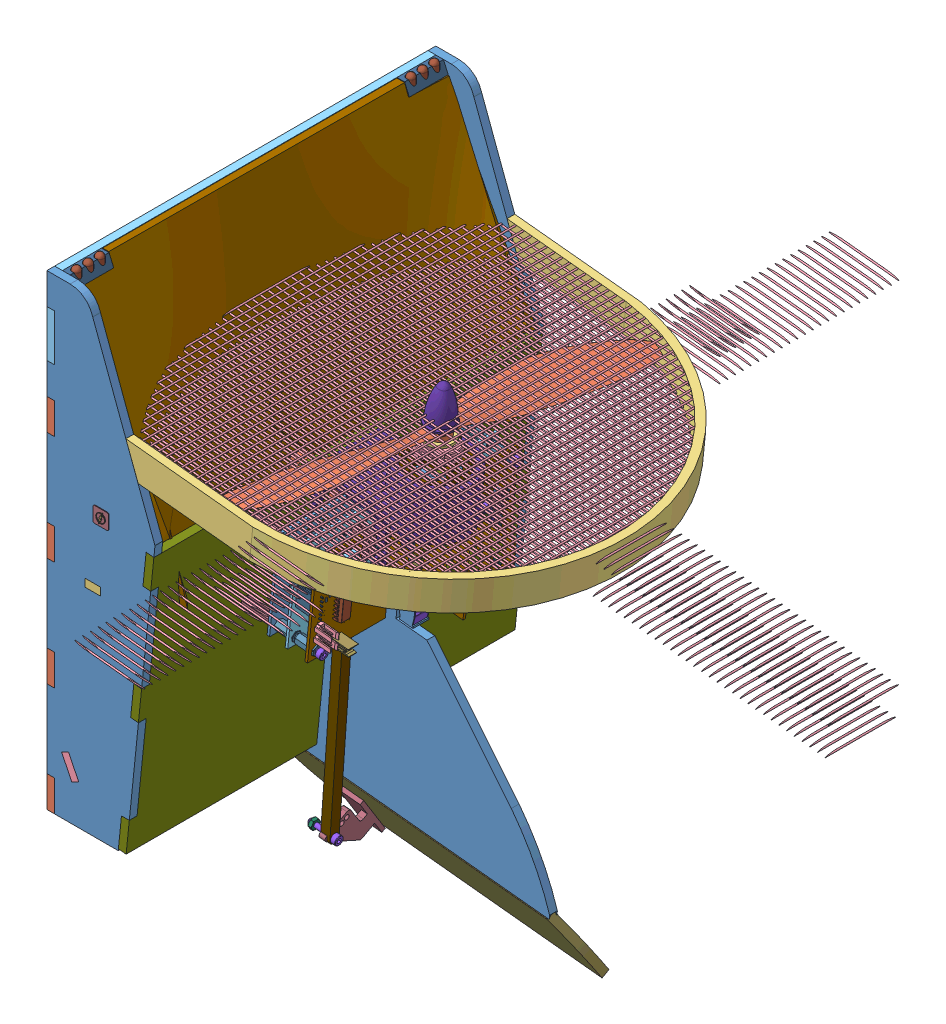
SolidWorks assembly AssTotaleSimu3, configuration Défaut. Lengths in mm. (continued)
Components (placement in the parent): (continued)
- AssStructSimu-1: AssStructSimu [Défaut] at (-125.7658 -1.8483 624.6548) x (1 0 0) z (0 0 -1) size (253.25 324.59 251.6) (continued)
  - AssCarte-1: AssCarte [Défaut] at (38.0121 147.1029 290.772) x (-0.101852 0.9948 0) z (0.9948 0.101852 0) size (66.52 130.57 98.72) (continued)
    - AssEntretoise-3: AssEntretoise [Défaut] at (-106.8199 -51.2976 37.1344) x (0 0 -1) z (1 0 0) size (58.24 7.29 7.81)
      - socket head cap screw 4762_din-1: socket head cap screw 4762_din [EN ISO 4762 M3 x 5 - 5N] at (-2.4967 0.5867 0) size (8 5.5 5.5)
      - hexagonal_spacer_MF_M3_H20_HEX5.5_FTD6_MTL6-1: hexagonal_spacer_MF_M3_H20_HEX5.5_FTD6_MTL6 [Défaut] at (48.3433 0.5867 0) x (0 0 1) z (-1 0 0) size (6.36 5.51 26)
      - hex nut style 1 gradeab_din-1: hex nut style 1 gradeab_din [Hexagon Nut ISO 4032 - M3 - W - N] at (53.3433 0.5867 0) x (0 0.943962 0.330053) z (-1 0 0) size (5.5 6.35 2.4)
      - hexagonal_spacer_MF_M3_H12_HEX5.5_FTD6_MTL6-2: hexagonal_spacer_MF_M3_H12_HEX5.5_FTD6_MTL6 [Défaut] at (27.0633 0.5867 0) x (0 0.248308 0.968681) z (-1 0 0) size (6.36 5.51 18)
      - hexagonal_spacer_MF_M3_H12_HEX5.5_FTD6_MTL6-3: hexagonal_spacer_MF_M3_H12_HEX5.5_FTD6_MTL6 [Défaut] at (13.7833 0.5867 0) x (0 0 1) z (-1 0 0) size (6.36 5.51 18)
    - AssEntretoise-4: AssEntretoise [Défaut] at (-106.8199 68.7024 37.1344) x (0 0 -1) z (1 0 0) size (58.24 7.29 7.81)
      - socket head cap screw 4762_din-1: socket head cap screw 4762_din [EN ISO 4762 M3 x 5 - 5N] at (-2.4967 0.5867 0) size (8 5.5 5.5)
      - hexagonal_spacer_MF_M3_H20_HEX5.5_FTD6_MTL6-1: hexagonal_spacer_MF_M3_H20_HEX5.5_FTD6_MTL6 [Défaut] at (48.3433 0.5867 0) x (0 0 1) z (-1 0 0) size (6.36 5.51 26)
      - hex nut style 1 gradeab_din-1: hex nut style 1 gradeab_din [Hexagon Nut ISO 4032 - M3 - W - N] at (53.3433 0.5867 0) x (0 0.943962 0.330053) z (-1 0 0) size (5.5 6.35 2.4)
      - hexagonal_spacer_MF_M3_H12_HEX5.5_FTD6_MTL6-2: hexagonal_spacer_MF_M3_H12_HEX5.5_FTD6_MTL6 [Défaut] at (27.0633 0.5867 0) x (0 0.248308 0.968681) z (-1 0 0) size (6.36 5.51 18)
      - hexagonal_spacer_MF_M3_H12_HEX5.5_FTD6_MTL6-3: hexagonal_spacer_MF_M3_H12_HEX5.5_FTD6_MTL6 [Défaut] at (13.7833 0.5867 0) x (0 0 1) z (-1 0 0) size (6.36 5.51 18)
    - AssMpu-1: AssMpu [Défaut] at (-150.6881 40.5798 29.6372) x (0.908747 0.417347 0) z (0 0 1) size (8 8 22.28)
      - hex nut style 1 gradeab_din-1: hex nut style 1 gradeab_din [Hexagon Nut ISO 4032 - M3 - W - N] at (0.2783 0.3227 1.2) size (5.5 6.35 2.4)
      - plain washer 6903 type ab_din-1: plain washer 6903 type ab_din [DIN 6903-A3] at (0.2783 0.3227 1.2) x (0 0 1) z (-1 0 0) size (1 8 8)
      - socket head cap screw 4762_din-1: socket head cap screw 4762_din [EN ISO 4762 M3 x 5 - 5N] at (0.2783 0.3227 19.76) x (0 0 -1) z (-0.852155 0.523289 0) size (8 5.5 5.5)
      - hexagonal_spacer_MF_M3_H12_HEX5.5_FTD6_MTL6-1: hexagonal_spacer_MF_M3_H12_HEX5.5_FTD6_MTL6 [Défaut] at (0.2783 0.3227 3.48) size (6.36 5.51 18)
    - AssMpu-2: AssMpu [Défaut] at (-130.3481 40.6665 29.6372) size (8 8 22.28)
      - hex nut style 1 gradeab_din-1: hex nut style 1 gradeab_din [Hexagon Nut ISO 4032 - M3 - W - N] at (0.2783 0.3227 1.2) size (5.5 6.35 2.4)
      - plain washer 6903 type ab_din-1: plain washer 6903 type ab_din [DIN 6903-A3] at (0.2783 0.3227 1.2) x (0 0 1) z (-1 0 0) size (1 8 8)
      - socket head cap screw 4762_din-1: socket head cap screw 4762_din [EN ISO 4762 M3 x 5 - 5N] at (0.2783 0.3227 19.76) x (0 0 -1) z (-0.852155 0.523289 0) size (8 5.5 5.5)
      - hexagonal_spacer_MF_M3_H12_HEX5.5_FTD6_MTL6-1: hexagonal_spacer_MF_M3_H12_HEX5.5_FTD6_MTL6 [Défaut] at (0.2783 0.3227 3.48) size (6.36 5.51 18)
    - AssCosse-1: AssCosse [Défaut] at (-142.6764 26.8797 71.168) x (0 -1 0) z (-0.344896 0 -0.938641) size (9.83 18.66 11.64)
      - socket head cap screw 4762_din-1: socket head cap screw 4762_din [EN ISO 4762 M3 x 6 - 6N] at (-5.1064 0.3659 0) size (9 5.5 5.5)
      - plain washer 6903 type ab_din-1: plain washer 6903 type ab_din [DIN 6903-A3] at (-2.1064 0.3659 0) size (1 8 8)
      - hex nut style 1 gradeab_din-2: hex nut style 1 gradeab_din [Hexagon Nut ISO 4032 - M3 - W - N] at (1.281 0.3659 0) x (0 0.924225 0.381849) z (-1 0 0) size (5.5 6.35 2.4)
      - 31880-1: 31880 [Default] at (0.4936 0.3659 0) x (0 0.344896 -0.938641) z (0 -0.938641 -0.344896) size (5.54 5 17.37)
    - AssCosse-2: AssCosse [Défaut] at (-142.6764 -2.9203 71.168) x (0 -1 0) z (-0.344896 0 -0.938641) size (9.83 18.66 11.64)
      - socket head cap screw 4762_din-1: socket head cap screw 4762_din [EN ISO 4762 M3 x 6 - 6N] at (-5.1064 0.3659 0) size (9 5.5 5.5)
      - plain washer 6903 type ab_din-1: plain washer 6903 type ab_din [DIN 6903-A3] at (-2.1064 0.3659 0) size (1 8 8)
      - hex nut style 1 gradeab_din-2: hex nut style 1 gradeab_din [Hexagon Nut ISO 4032 - M3 - W - N] at (1.281 0.3659 0) x (0 0.924225 0.381849) z (-1 0 0) size (5.5 6.35 2.4)
      - 31880-1: 31880 [Default] at (0.4936 0.3659 0) x (0 0.344896 -0.938641) z (0 -0.938641 -0.344896) size (5.54 5 17.37)
    - AssCosse-3: AssCosse [Défaut] at (-142.6764 12.0797 71.168) x (0 -1 0) z (-0.344896 0 -0.938641) size (9.83 18.66 11.64)
      - socket head cap screw 4762_din-1: socket head cap screw 4762_din [EN ISO 4762 M3 x 6 - 6N] at (-5.1064 0.3659 0) size (9 5.5 5.5)
      - plain washer 6903 type ab_din-1: plain washer 6903 type ab_din [DIN 6903-A3] at (-2.1064 0.3659 0) size (1 8 8)
      - hex nut style 1 gradeab_din-2: hex nut style 1 gradeab_din [Hexagon Nut ISO 4032 - M3 - W - N] at (1.281 0.3659 0) x (0 0.924225 0.381849) z (-1 0 0) size (5.5 6.35 2.4)
      - 31880-1: 31880 [Default] at (0.4936 0.3659 0) x (0 0.344896 -0.938641) z (0 -0.938641 -0.344896) size (5.54 5 17.37)
    - Terminal_QD_Female-1: Terminal_QD_Female [Default] at (-137.2199 31.5422 53.3942) x (0 1 0) z (-1 0 0) size (9.4 5.5 22.35)
    - Terminal_QD_Female-2: Terminal_QD_Female [Default] at (-137.3199 31.5422 36.2942) x (0 -1 0) z (-1 0 0) size (9.4 5.5 22.35)
    - Terminal_QD_Female-3: Terminal_QD_Female [Default] at (-137.2199 1.7422 53.3942) x (0 1 0) z (-1 0 0) size (9.4 5.5 22.35)
    - Terminal_QD_Female-4: Terminal_QD_Female [Default] at (-137.3199 1.7422 35.9942) x (0 1 0) z (-1 0 0) size (9.4 5.5 22.35)
    - Terminal_QD_Female-5: Terminal_QD_Female [Default] at (-137.3199 16.7422 35.9942) x (0 1 0) z (-1 0 0) size (9.4 5.5 22.35)
    - Terminal_QD_Female-6: Terminal_QD_Female [Default] at (-137.2199 16.7422 53.3942) x (0 1 0) z (-1 0 0) size (9.4 5.5 22.35)
- AssTige-1: AssTige [Défaut] at (-241.576 -121.7726 340.4233) x (-0.101791 -0.994204 -0.034587) z (0.9948 -0.101852 0) size (166.39 7.19 19)
  - tige_servo-1: tige_servo [Défaut] at (-106.2712 0.2685 162) size (165 6 6)
  - socket head cap screw 4762_din-2: socket head cap screw 4762_din [EN ISO 4762 M2 x 10 - 10N] at (-104.2712 3.2685 170) x (0 0 -1) z (0.923728 0.383049 0) size (12 3.8 3.8)
  - hex nut style 1 gradeab_din-1: hex nut style 1 gradeab_din [Hexagon Nut ISO 4032 - M3 - W - N] at (55.7288 3.2685 156) size (5.5 6.35 2.4)
  - hex nut style 1 gradeab_din-2: hex nut style 1 gradeab_din [Hexagon Nut ISO 4032 - M2 - W - N] at (-104.2712 3.2685 160) x (0.904801 0.425836 0) z (0 0 1) size (4 4.62 1.6)
  - socket head cap screw 4762_din-3: socket head cap screw 4762_din [EN ISO 4762 M3 x 16 - 16N] at (55.7288 3.2685 171) x (0 0 -1) z (0.923728 0.383049 0) size (19 5.5 5.5)
- AssGoPro-1: AssGoPro [Défaut] at (-119.9926 15.1708 318.2917) x (0 0 -1) z (-0.119031 -0.99289 0) size (64.3 52.3 34.42)
  - GoPRo Frame for LCD Screen-1: GoPRo Frame for LCD Screen [Défaut] at (-2.6935 10.9558 5.5635) size (64.3 59.3 34.42)
    - GoProFrame MJM-1: GoProFrame MJM [Défaut] at (-3.6084 -1.6692 52.45) size (64.3 59.3 23.5)
    - GoPro Hero 3 Front Panel-1: GoPro Hero 3 Front Panel [Défaut] at (-3.6084 -1.6692 55.7) x (-1 0 0) z (0 0 -1) size (59.25 41.2 1.9)
    - GoPro Hero 3 Screen-1: GoPro Hero 3 Screen [Défaut] at (12.7166 3.9308 54.9) size (15 18 1)
    - GoPro Hero 3 Mode Button-1: GoPro Hero 3 Mode Button [Défaut] at (13.4166 -12.4692 54.95) x (-1 0 0) z (0 0 -1) size (11.97 12.11 3.03)
    - GoPro Hero 3 LED Cover-1: GoPro Hero 3 LED Cover [Défaut] at (3.1166 -9.3192 54.85) x (-0.999988 0.004848 0) z (0 0 -1) size (5 5 1.4)
    - GoPro Hero 3 LED Cover-2: GoPro Hero 3 LED Cover [Défaut] at (3.1166 -16.0692 54.85) x (-0.999988 0.004848 0) z (0 0 -1) size (5 5 1.4)
    - GoPro Hero 3 Housing-1: GoPro Hero 3 Housing [Défaut] at (-3.6084 -1.6692 55.7) size (59.37 41.3 29.84)
    - GoPro Hero 3 Lens-1: GoPro Hero 3 Lens [Défaut] at (-18.9334 5.6308 47.35) x (-0.380542 -0.924764 0) z (0 0 -1) size (13.71 15.7 7.94)
    - GoPro Hero 3 Indicator Cover-1: GoPro Hero 3 Indicator Cover [Défaut] at (-25.5834 -22.2692 69.9) x (-0.997412 0 -0.0719) z (0 1 0) size (3 3 2)
    - GoPro Hero 3 Indicator Cover-2: GoPro Hero 3 Indicator Cover [Défaut] at (-28.8834 12.2308 73) x (-0.999992 0.004018 0) z (0 0 1) size (3 3 2)
    - GoPro Hero 3 Indicator Cover-3: GoPro Hero 3 Indicator Cover [Défaut] at (20.6666 16.9308 58.4) x (-0.997739 0 -0.067212) z (0 1 0) size (3 3 2)
    - slot-1: slot [Défaut] at (-24.7434 -9.7363 65.05) x (0 1 0) z (0 0 -1) size (16 15.02 2.44)
    - GoPro Hero 3 HDMI pin-1: GoPro Hero 3 HDMI pin [Défaut] at (-26.982 2.9815 24.7172) x (0.105491 0.98175 -0.158237) z (-0.992872 0.095109 -0.071829) size (3.29 0.86 3.28)
  - support1-2: support1 [Défaut] at (-1.3019 -18.8633 67.0135) x (0 0 1) z (-1 0 0) size (5 5 10)
- AssGouv-1: AssGouv [Défaut] at (-43.2668 -298.2106 479.8345) x (0.9948 -0.101852 0) z (0.055947 0.546439 -0.835628) size (200.18 52.5 43.47)
  - P10_1-1: P10_1 [Défaut] at (-108.1667 -19.4144 197.6829) size (200.18 50.13 5)
  - attache_pale-1: attache_pale [Défaut] at (-49.1667 8.0856 190.1829) x (0 0 -1) z (-1 0 0) size (43.47 35 14)
- Parallax-Servo-Horn-1: Parallax-Servo-Horn [Défaut] at (-69.3162 -29.8353 324.5606) x (0.09792 0.956393 0.27518) z (0.9948 -0.101852 0) size (38.81 38.81 6.17)
- NTM_35-36_engine_assembly-1: NTM_35-36_engine_assembly [Défaut] at (-24.3523 26.8781 325.7101) x (0.9948 -0.101852 0) z (0 0 1) size (60.56 77.2 246.41)
  - engine_base-1: engine_base [Défaut] at (-1.8719 -19.5526 -1.1165) x (0 1 0) z (0 0 1) size (6.8 35 35)
  - engine_bearing-1: engine_bearing [Défaut] at origin size (10 4 10)
  - Propeller_cone-1: Propeller_cone [Défaut] at (-1.8719 33.6474 -4.1165) x (1 0 0) z (0 1 0) size (17.6 17.6 24)
  - engine_bearing-2: engine_bearing [Défaut] at (0 22.8 0) size (10 4 10)
  - NTM_35-36_enginebody-1: NTM_35-36_enginebody [Défaut] at (-1.8719 -12.7526 -1.1165) size (35 31.7 35)
  - Stator-1: Stator [Défaut] at origin size (27.75 22.36 27.94)
  - propellers_10x4-1: propellers_10x4 [Défaut] at (-6.8719 27.4474 -4.9165) size (60.56 10.53 246.41)
  - propeller_washer-1: propeller_washer [Défaut] at (-1.8719 24.4474 -1.1165) x (0 1 0) z (0 0 1) size (2.5 18 18)
  - Propeller_adaptor-1: Propeller_adaptor [Défaut] at (2.1948 17.1101 -3.713) size (23.46 32.5 25)
Mates (geometry in assembly coordinates):
- Coaxiale1: concentric aligned: cylinder of AssStructSimu-1/AssToitMot-1/AssToit-1/P12-1 through (-27.6967 12.5918 324.5936) axis (-0.101852 -0.9948 0) radius 17.5; cylinder of NTM_35-36_engine_assembly-1/NTM_35-36_enginebody-1 through (-25.2217 36.7654 324.5936) axis (-0.101852 -0.9948 0) radius 17.5
- Coïncidente1: coincident anti-aligned: plane of AssStructSimu-1/AssToitMot-1/AssToit-1/P12-1 through (-28.206 7.6178 324.5936) normal (0.101852 0.9948 0); plane of NTM_35-36_engine_assembly-1/engine_bearing-1 through (-28.206 7.6178 324.5936) normal (-0.101852 -0.9948 0)
- Coaxiale2: concentric aligned: cylinder of AssStructSimu-1/AssToitMot-1/AssToit-1/P10_2-1 through (49.7135 -178.7878 324.5936) axis (-0.9948 0.101852 0) radius 2.5; cylinder of AssGouv-1/P10_1-1 through (-94.0351 -164.0702 324.5936) axis (-0.9948 0.101852 0) radius 2.5
- Coïncidente2: coincident aligned: plane of AssStructSimu-1/AssToitMot-1/AssToit-1/P10_2-1 through (-137.5516 -157.1017 322.0936) normal (-0.9948 0.101852 0); plane of AssGouv-1/P10_1-1 through (-137.8791 -160.3008 321.1312) normal (-0.9948 0.101852 0)
- Coaxiale3: concentric aligned: cylinder of AssTige-1/socket head cap screw 4762_din-3 through (-45.5416 -197.7164 335.2292) axis (0.9948 -0.101852 0) radius 1.5; cylinder of AssGouv-1/attache_pale-1 through (-85.9983 -193.5742 335.2292) axis (0.9948 -0.101852 0) radius 1.5
- Coaxiale4: concentric aligned: cylinder of AssStructSimu-1/AssToitMot-1/Parallax-Servo_DUMMY-1 through (-70.6554 -29.6982 324.5606) axis (-0.9948 0.101852 0) radius 2.9845; cylinder of Parallax-Servo-Horn-1 through (-70.6554 -29.6982 324.5606) axis (-0.9948 0.101852 0) radius 2.9845
- Coïncidente3: coincident anti-aligned: plane of AssStructSimu-1/AssToitMot-1/Parallax-Servo_DUMMY-1 through (-74.8246 -29.2713 324.5606) normal (0.9948 -0.101852 0); plane of Parallax-Servo-Horn-1 through (-74.8246 -29.2713 324.5606) normal (-0.9948 0.101852 0)
- Coaxiale5: concentric anti-aligned: cylinder of AssTige-1/socket head cap screw 4762_din-2 through (-30.2498 -38.5418 340.7631) axis (0.9948 -0.101852 0) radius 1; cylinder of Parallax-Servo-Horn-1 through (-69.7931 -34.4932 340.7631) axis (-0.9948 0.101852 0) radius 0.635
- Coïncidente4: coincident anti-aligned: plane of AssTige-1/tige_servo-1 through (-69.6001 -32.608 343.8305) normal (-0.9948 0.101852 0); plane of Parallax-Servo-Horn-1 through (-68.8748 -25.5237 332.3708) normal (0.9948 -0.101852 0)
- Coaxiale6: concentric aligned: cylinder of AssStructSimu-1/AssBase-1/socket head cap screw 4762_din-7 through (-144.5139 -51.9008 369.3436) axis (0 0 1) radius 1.5; cylinder of AssGoPro-1/support1-2 through (-144.5139 -51.9008 319.5936) axis (0 0 1) radius 1.5
- Coïncidente5: coincident anti-aligned: plane of AssStructSimu-1/AssBase-1/support2-1 through (-141.9706 -54.3568 329.5936) normal (0 0 -1); plane of AssGoPro-1/support1-2 through (-146.6985 -49.121 329.5936) normal (0 0 1)
